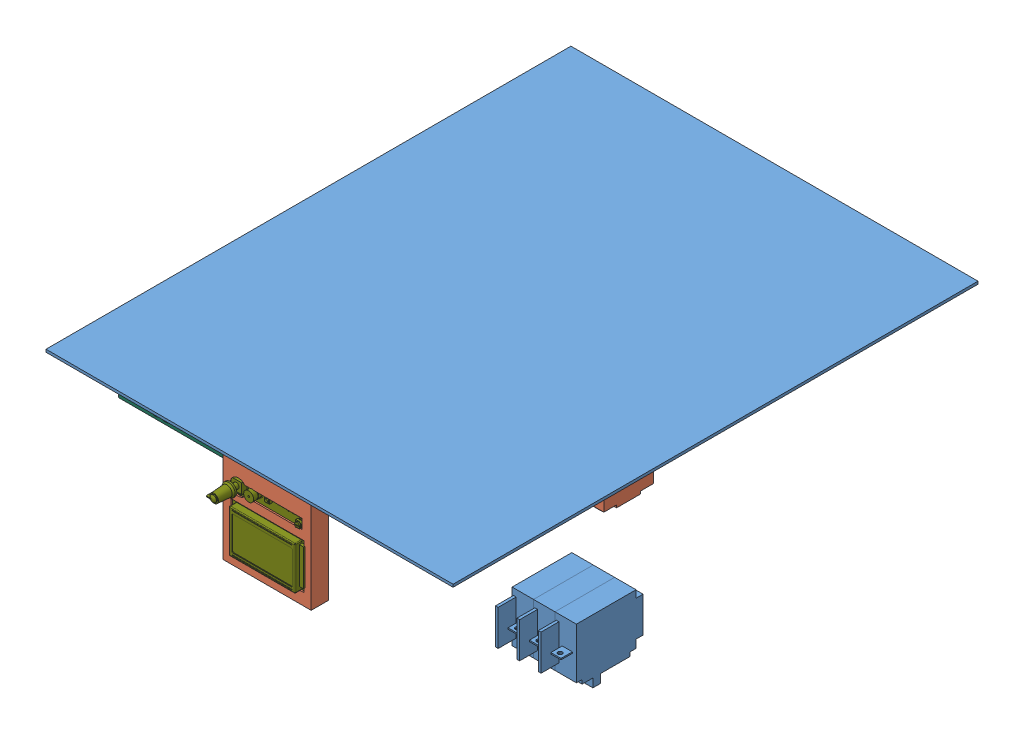
SolidWorks assembly CASE ASSEMBLY, configuration Default. Lengths in mm. (continued)
Components (placement in the parent): (continued)
- BIGTREETECH SKR 2-3D.step-2: BIGTREETECH SKR 2-3D.step [Default] at (122.8656 -8.0191 -250.7922) x (0 0 1) z (0 -1 0) size (112.33 85.75 22.11) (continued)
  - R42.step-1: R42.step [Default] at origin size (1.6 0.8 0.45)
    - R0603.step-1: R0603.step [Default] at (391.1973 179.6035 0) x (1 0 0) z (0 0 1) size (1.6 0.8 0.45)
  - R46.step-1: R46.step [Default] at origin size (0.8 1.6 0.45)
    - R0603.step-1: R0603.step [Default] at (425.1768 173.2653 0) x (0 1 0) z (0 0 1) size (1.6 0.8 0.45)
  - R48.step-1: R48.step [Default] at origin size (1.6 0.8 0.45)
    - R0603.step-1: R0603.step [Default] at (402.9463 182.6842 0) x (1 0 0) z (0 0 1) size (1.6 0.8 0.45)
  - R49.step-1: R49.step [Default] at origin size (0.8 1.6 0.45)
    - R0603.step-1: R0603.step [Default] at (446.7668 160.3113 0) x (0 1 0) z (0 0 1) size (1.6 0.8 0.45)
  - R50.step-1: R50.step [Default] at origin size (0.8 1.6 0.45)
    - R0603.step-1: R0603.step [Default] at (433.2882 166.9697 0) x (0 -1 0) z (0 0 1) size (1.6 0.8 0.45)
  - R52.step-1: R52.step [Default] at origin size (0.8 1.6 0.45)
    - R0603.step-1: R0603.step [Default] at (434.7018 167.0423 0) x (0 1 0) z (0 0 1) size (1.6 0.8 0.45)
  - R53.step-1: R53.step [Default] at origin size (0.8 1.6 0.45)
    - R0603.step-1: R0603.step [Default] at (446.7668 163.3593 0) x (0 1 0) z (0 0 1) size (1.6 0.8 0.45)
  - R54.step-1: R54.step [Default] at origin size (1.6 0.8 0.45)
    - R0603.step-1: R0603.step [Default] at (433.9247 169.8598 0) x (-1 0 0) z (0 0 1) size (1.6 0.8 0.45)
  - R56.step-1: R56.step [Default] at origin size (1.6 0.8 0.45)
    - R0603.step-1: R0603.step [Default] at (433.5407 202.6728 0) x (-1 0 0) z (0 0 1) size (1.6 0.8 0.45)
  - R57.step-1: R57.step [Default] at origin size (1.6 0.8 0.45)
    - R0603.step-1: R0603.step [Default] at (446.2067 202.0128 0) x (-1 0 0) z (0 0 1) size (1.6 0.8 0.45)
  - R58.step-1: R58.step [Default] at origin size (1.6 0.8 0.45)
    - R0603.step-1: R0603.step [Default] at (433.5087 201.1282 0) x (-1 0 0) z (0 0 1) size (1.6 0.8 0.45)
  - R59.step-1: R59.step [Default] at origin size (1.6 0.8 0.45)
    - R0603.step-1: R0603.step [Default] at (446.2816 200.6068 0) x (1 0 0) z (0 0 1) size (1.6 0.8 0.45)
  - R60.step-1: R60.step [Default] at origin size (1.6 0.8 0.45)
    - R0603.step-1: R0603.step [Default] at (398.6873 207.4379 0) x (1 0 0) z (0 0 1) size (1.6 0.8 0.45)
  - R61.step-1: R61.step [Default] at origin size (1.6 0.8 0.45)
    - R0603.step-1: R0603.step [Default] at (402.6377 207.2995 0) x (-1 0 0) z (0 0 1) size (1.6 0.8 0.45)
  - R62.step-1: R62.step [Default] at origin size (1.6 0.8 0.45)
    - R0603.step-1: R0603.step [Default] at (433.5027 199.6398 0) x (-1 0 0) z (0 0 1) size (1.6 0.8 0.45)
  - R64.step-1: R64.step [Default] at origin size (1.6 0.8 0.45)
    - R0603.step-1: R0603.step [Default] at (402.7123 205.8629 0) x (1 0 0) z (0 0 1) size (1.6 0.8 0.45)
  - R70.step-1: R70.step [Default] at origin size (1.6 0.8 0.45)
    - R0603.step-1: R0603.step [Default] at (398.8373 198.8192 0) x (1 0 0) z (0 0 1) size (1.6 0.8 0.45)
  - R71.step-1: R71.step [Default] at origin size (1.6 0.8 0.45)
    - R0603.step-1: R0603.step [Default] at (402.9123 198.7442 0) x (1 0 0) z (0 0 1) size (1.6 0.8 0.45)
  - R73.step-1: R73.step [Default] at origin size (1.6 0.8 0.45)
    - R0603.step-1: R0603.step [Default] at (402.9373 197.2645 0) x (1 0 0) z (0 0 1) size (1.6 0.8 0.45)
  - R75.step-1: R75.step [Default] at origin size (1.6 0.8 0.45)
    - R0603.step-1: R0603.step [Default] at (414.6557 183.6875 0) x (1 0 0) z (0 0 1) size (1.6 0.8 0.45)
  - R76.step-1: R76.step [Default] at origin size (1.6 0.8 0.45)
    - R0603.step-1: R0603.step [Default] at (417.6657 183.6228 0) x (-1 0 0) z (0 0 1) size (1.6 0.8 0.45)
  - R78.step-1: R78.step [Default] at origin size (1.6 0.8 0.45)
    - R0603.step-1: R0603.step [Default] at (417.6657 185.1468 0) x (-1 0 0) z (0 0 1) size (1.6 0.8 0.45)
  - R79.step-1: R79.step [Default] at origin size (1.6 0.8 0.45)
    - R0603.step-1: R0603.step [Default] at (410.1103 163.3762 0) x (1 0 0) z (0 0 1) size (1.6 0.8 0.45)
  - R80.step-1: R80.step [Default] at origin size (0.8 1.6 0.45)
    - R0603.step-1: R0603.step [Default] at (410.8445 159.5197 0) x (0 -1 0) z (0 0 1) size (1.6 0.8 0.45)
  - R81.step-1: R81.step [Default] at origin size (1.6 0.8 0.45)
    - R0603.step-1: R0603.step [Default] at (414.9294 190.8632 0) x (1 0 0) z (0 0 1) size (1.6 0.8 0.45)
  - R82.step-1: R82.step [Default] at origin size (1.6 0.8 0.45)
    - R0603.step-1: R0603.step [Default] at (418.3337 195.4355 0) x (-1 0 0) z (0 0 1) size (1.6 0.8 0.45)
  - R83.step-1: R83.step [Default] at origin size (0.8 1.6 0.45)
    - R0603.step-1: R0603.step [Default] at (409.3632 159.5197 0) x (0 -1 0) z (0 0 1) size (1.6 0.8 0.45)
  - R84.step-1: R84.step [Default] at origin size (1.6 0.8 0.45)
    - R0603.step-1: R0603.step [Default] at (418.3337 193.9418 0) x (-1 0 0) z (0 0 1) size (1.6 0.8 0.45)
  - U4.step-1: U4.step [Default] at origin size (6.2 5 1.75)
    - HSOP8.step-1: HSOP8.step [Default] at (423.1921 177.6994 0) x (1 0 0) z (0 -1 0) size (6.2 1.75 5)
      - Assy_fuss_hsop8_____________.step-1: Assy_fuss_hsop8_____________.step [Default] at (2 0 0) size (1.1 0.95 4.25)
        - Fuss_hsop8_____________.step-1: Fuss_hsop8_____________.step [Default] at (0 0 -0.635) size (1.1 0.95 0.44)
        - Fuss_hsop8_____________.step-2: Fuss_hsop8_____________.step [Default] at (0 0 0.635) size (1.1 0.95 0.44)
        - Fuss_hsop8_____________.step-3: Fuss_hsop8_____________.step [Default] at (0 0 1.905) size (1.1 0.95 0.44)
        - Fuss_hsop8_____________.step-4: Fuss_hsop8_____________.step [Default] at (0 0 -1.905) size (1.1 0.95 0.44)
        - Fuss_hsop8_____________.step-5: Fuss_hsop8_____________.step [Default] at (0 0 -0.635) size (1.1 0.95 0.44)
        - Fuss_hsop8_____________.step-6: Fuss_hsop8_____________.step [Default] at (0 0 0.635) size (1.1 0.95 0.44)
      - Assy_fuss_hsop8_____________-1.step-1: Assy_fuss_hsop8_____________-1.step [Default] at (-2 0 0) x (-1 0 0) z (0 0 -1) size (1.1 0.95 4.25)
        - Fuss_hsop8_____________.step-1: Fuss_hsop8_____________.step [Default] at (0 0 -0.635) size (1.1 0.95 0.44)
        - Fuss_hsop8_____________.step-2: Fuss_hsop8_____________.step [Default] at (0 0 0.635) size (1.1 0.95 0.44)
        - Fuss_hsop8_____________.step-3: Fuss_hsop8_____________.step [Default] at (0 0 1.905) size (1.1 0.95 0.44)
        - Fuss_hsop8_____________.step-4: Fuss_hsop8_____________.step [Default] at (0 0 -1.905) size (1.1 0.95 0.44)
        - Fuss_hsop8_____________.step-5: Fuss_hsop8_____________.step [Default] at (0 0 -0.635) size (1.1 0.95 0.44)
        - Fuss_hsop8_____________.step-6: Fuss_hsop8_____________.step [Default] at (0 0 0.635) size (1.1 0.95 0.44)
      - part_hsop8_____________.step-1: part_hsop8_____________.step [Default] at origin size (4 1.75 5)
  - F1.step-1: F1.step [Default] at origin size (3.48 4.74 1.03)
    - Fuse_1812.step-1: Fuse_1812.step [Default] at (437.3627 175.895 0) x (0 -1 0) z (0 0 1) size (4.73 3.48 1.03)
  - Probe.step-1: Probe.step [Default] at origin size (8 6 11)
    - User_Library-XH2_54_2PIN_RGB0.step-1: User_Library-XH2_54_2PIN_RGB0.step [Default] at (488.1051 165.2532 0) x (-1 0 0) z (0 1 0) size (8 11 6)
  - P1.step-1: P1.step [Default] at origin size (15.24 5.85 7.5)
    - 810112480.step-1: 810112480.step [Default] at (479.9341 168.4042 0) size (15.24 5.84 6)
      - Extruded-31.step-1: Extruded-31.step [Default] at origin size (15.24 5.84 6)
    - 810111120.step-1: 810111120.step [Default] at (485.5337 171.1537 0) size (1.02 0.36 2.4)
      - Extruded-3.step-1: Extruded-3.step [Default] at origin size (1.02 0.36 2.4)
    - 810112616.step-1: 810112616.step [Default] at (480.2983 171.1537 0) size (9.38 0.36 6)
      - Extruded-32.step-1: Extruded-32.step [Default] at origin size (9.38 0.36 6)
    - 810112752.step-1: 810112752.step [Default] at (479.972 168.3823 0) size (14.76 5.32 0.5)
      - Extruded-33.step-1: Extruded-33.step [Default] at origin size (14.76 5.32 0.5)
    - 860059712.step-1: 860059712.step [Default] at (477.402 168.7861 -1.5) x (0 1 0) z (0 0 1) size (1 1 6)
      - Cylinder.step-1: Cylinder.step [Default] at origin size (1 1 6)
    - 860059712.step-2: 860059712.step [Default] at (479.942 168.7861 -1.5) x (0 1 0) z (0 0 1) size (1 1 6)
      - Cylinder.step-1: Cylinder.step [Default] at origin size (1 1 6)
    - 860059712.step-3: 860059712.step [Default] at (482.482 168.7861 -1.5) x (0 1 0) z (0 0 1) size (1 1 6)
      - Cylinder.step-1: Cylinder.step [Default] at origin size (1 1 6)
    - 860059712.step-4: 860059712.step [Default] at (485.022 168.7861 -1.5) x (0 1 0) z (0 0 1) size (1 1 6)
      - Cylinder.step-1: Cylinder.step [Default] at origin size (1 1 6)
    - 810110576.step-1: 810110576.step [Default] at (475.101 171.1382 0) size (1.02 0.37 2.4)
      - Extruded.step-1: Extruded.step [Default] at origin size (1.02 0.37 2.4)
    - 860060864.step-1: 860060864.step [Default] at (474.856 168.9105 0) x (-1 0 0) z (0 0 1) size (1 1 4.5)
      - Cylinder-34.step-1: Cylinder-34.step [Default] at origin size (1 1 4.5)
  - R88.step-1: R88.step [Default] at origin size (1.6 0.8 0.45)
    - R0603.step-1: R0603.step [Default] at (464.0563 185.2452 0) x (1 0 0) z (0 0 1) size (1.6 0.8 0.45)
  - R89.step-1: R89.step [Default] at origin size (1.6 0.8 0.45)
    - R0603.step-1: R0603.step [Default] at (464.0563 186.7202 0) x (1 0 0) z (0 0 1) size (1.6 0.8 0.45)
  - R90.step-1: R90.step [Default] at origin size (1.6 0.8 0.45)
    - R0603.step-1: R0603.step [Default] at (464.0563 188.1952 0) x (1 0 0) z (0 0 1) size (1.6 0.8 0.45)
  - D14.step-1: D14.step [Default] at origin size (1.61 0.81 0.61)
    - LED_0603_G.step-1: LED_0603_G.step [Default] at (443.6801 162.0518 0) x (-1 0 0) z (0 0 1) size (1.61 0.81 0.61)
      - User_Library-LED_0603_G_Pocket002.step-1: User_Library-LED_0603_G_Pocket002.step [Default] at origin size (0.41 0.81 0.21)
      - User_Library-LED_0603_G_Pad004.step-1: User_Library-LED_0603_G_Pad004.step [Default] x (1 0 0) z (0 0 -1) size (0.4 0.8 0)
      - User_Library-LED_0603_G_Fillet.step-1: User_Library-LED_0603_G_Fillet.step [Default] at origin size (1 0.7 0.4)
      - User_Library-LED_0603_G_Pocket001.step-1: User_Library-LED_0603_G_Pocket001.step [Default] at origin size (0.4 0.8 0.2)
      - User_Library-LED_0603_G_Pad.step-1: User_Library-LED_0603_G_Pad.step [Default] at origin size (0.8 0.8 0.2)
  - C21.step-1: C21.step [Default] at origin size (1.6 0.8 0.8)
    - 810108944.step-1: 810108944.step [Default] at (458.6741 172.9827 0) size (1.14 0.8 0.8)
      - Extruded-22.step-1: Extruded-22.step [Default] at origin size (1.14 0.8 0.8)
    - 810108400.step-1: 810108400.step [Default] at (457.9891 172.9826 0) size (0.23 0.8 0.8)
      - Extruded-23.step-1: Extruded-23.step [Default] at origin size (0.23 0.8 0.8)
    - 810108400.step-2: 810108400.step [Default] at (459.3591 172.9826 0) size (0.23 0.8 0.8)
      - Extruded-23.step-1: Extruded-23.step [Default] at origin size (0.23 0.8 0.8)
  - C60.step-1: C60.step [Default] at origin size (2 1.25 0.78)
    - User_Library-0805_SMD_Capacitor.step-1: User_Library-0805_SMD_Capacitor.step [Default] at (458.5985 175.133 -0.01) x (1 0 0) z (0 -1 0) size (2 0.78 1.25)
  - C61.step-1: C61.step [Default] at origin size (0.81 1.6 0.8)
    - 810109216.step-1: 810109216.step [Default] at (458.0803 162.4211 0) size (0.8 1.14 0.8)
      - Extruded-11.step-1: Extruded-11.step [Default] at origin size (0.8 1.14 0.8)
    - 810109080.step-1: 810109080.step [Default] at (458.0804 161.7361 0) size (0.8 0.23 0.8)
      - Extruded-10.step-1: Extruded-10.step [Default] at origin size (0.8 0.23 0.8)
    - 810109080.step-2: 810109080.step [Default] at (458.0804 163.1061 0) size (0.8 0.23 0.8)
      - Extruded-10.step-1: Extruded-10.step [Default] at origin size (0.8 0.23 0.8)
  - C62.step-1: C62.step [Default] at origin size (1.6 0.8 0.8)
    - 810108944.step-1: 810108944.step [Default] at (463.8994 193.9377 0) size (1.14 0.8 0.8)
      - Extruded-22.step-1: Extruded-22.step [Default] at origin size (1.14 0.8 0.8)
    - 810108400.step-1: 810108400.step [Default] at (463.2144 193.9376 0) size (0.23 0.8 0.8)
      - Extruded-23.step-1: Extruded-23.step [Default] at origin size (0.23 0.8 0.8)
    - 810108400.step-2: 810108400.step [Default] at (464.5844 193.9376 0) size (0.23 0.8 0.8)
      - Extruded-23.step-1: Extruded-23.step [Default] at origin size (0.23 0.8 0.8)
  - C63.step-1: C63.step [Default] at origin size (0.8 1.6 0.8)
    - 810109216.step-1: 810109216.step [Default] at (448.5727 199.9859 0) size (0.8 1.14 0.8)
      - Extruded-11.step-1: Extruded-11.step [Default] at origin size (0.8 1.14 0.8)
    - 810109080.step-1: 810109080.step [Default] at (448.5726 200.6709 0) size (0.8 0.23 0.8)
      - Extruded-10.step-1: Extruded-10.step [Default] at origin size (0.8 0.23 0.8)
    - 810109080.step-2: 810109080.step [Default] at (448.5726 199.3009 0) size (0.8 0.23 0.8)
      - Extruded-10.step-1: Extruded-10.step [Default] at origin size (0.8 0.23 0.8)
  - D19.step-1: D19.step [Default] at origin size (1.61 0.81 0.61)
    - LED_0603_G.step-1: LED_0603_G.step [Default] at (414.9232 199.3538 0) x (-1 0 0) z (0 0 1) size (1.61 0.81 0.61)
      - User_Library-LED_0603_G_Pocket002.step-1: User_Library-LED_0603_G_Pocket002.step [Default] at origin size (0.41 0.81 0.21)
      - User_Library-LED_0603_G_Pad004.step-1: User_Library-LED_0603_G_Pad004.step [Default] x (1 0 0) z (0 0 -1) size (0.4 0.8 0)
      - User_Library-LED_0603_G_Fillet.step-1: User_Library-LED_0603_G_Fillet.step [Default] at origin size (1 0.7 0.4)
      - User_Library-LED_0603_G_Pocket001.step-1: User_Library-LED_0603_G_Pocket001.step [Default] at origin size (0.4 0.8 0.2)
      - User_Library-LED_0603_G_Pad.step-1: User_Library-LED_0603_G_Pad.step [Default] at origin size (0.8 0.8 0.2)
  - D20.step-1: D20.step [Default] at origin size (1.25 2.02 1.1)
    - User_Library-led_0805.step-1: User_Library-led_0805.step [Default] at (462.7879 175.6538 0) x (0 1 0) z (0 0 1) size (2.02 1.25 1.1)
  - J1.step-1: J1.step [Default] at origin size (12.7 2.54 11.54)
    - 1001-5.step-1: 1001-5.step [Default] at (468.874 170.561 0) x (-1 0 0) z (0 0 1) size (12.7 2.54 11.54)
  - P2.step-1: P2.step [Default] at origin size (5.08 7.62 11.54)
    - 1001-3.step-1: 1001-3.step [Default] at (452.9366 163.9727 0) x (0 1 0) z (0 0 1) size (7.62 2.54 11.54)
    - 1001-3.step-2: 1001-3.step [Default] at (455.4766 163.9727 0) x (0 1 0) z (0 0 1) size (7.62 2.54 11.54)
  - Q10.step-1: Q10.step [Default] at origin size (3 3 1.3)
    - 860057152.step-1: 860057152.step [Default] at (414.6295 201.7671 0) x (0 -1 0) z (-1 0 0) size (3 1.3 3)
  - R16.step-1: R16.step [Default] at origin size (1.6 0.8 0.45)
    - R0603.step-1: R0603.step [Default] at (465.2907 172.9548 0) x (-1 0 0) z (0 0 1) size (1.6 0.8 0.45)
  - R18.step-1: R18.step [Default] at origin size (0.8 1.6 0.45)
    - R0603.step-1: R0603.step [Default] at (461.2448 175.6724 0) x (0 1 0) z (0 0 1) size (1.6 0.8 0.45)
  - R19.step-1: R19.step [Default] at origin size (1.6 0.8 0.45)
    - R0603.step-1: R0603.step [Default] at (462.0633 172.9932 0) x (1 0 0) z (0 0 1) size (1.6 0.8 0.45)
  - R45.step-1: R45.step [Default] at origin size (1.6 0.8 0.45)
    - R0603.step-1: R0603.step [Default] at (455.7657 161.6518 0) x (-1 0 0) z (0 0 1) size (1.6 0.8 0.45)
  - R47.step-1: R47.step [Default] at origin size (1.6 0.8 0.45)
    - R0603.step-1: R0603.step [Default] at (452.7923 161.6902 0) x (1 0 0) z (0 0 1) size (1.6 0.8 0.45)
  - R85.step-1: R85.step [Default] at origin size (0.8 1.6 0.45)
    - R0603.step-1: R0603.step [Default] at (432.2065 162.8147 0) x (0 -1 0) z (0 0 1) size (1.6 0.8 0.45)
  - R92.step-1: R92.step [Default] at origin size (1.6 0.8 0.45)
    - R0603.step-1: R0603.step [Default] at (414.9294 197.8492 0) x (1 0 0) z (0 0 1) size (1.6 0.8 0.45)
  - R93.step-1: R93.step [Default] at origin size (1.6 0.8 0.45)
    - R0603.step-1: R0603.step [Default] at (418.2897 202.5098 0) x (-1 0 0) z (0 0 1) size (1.6 0.8 0.45)
  - R94.step-1: R94.step [Default] at origin size (1.6 0.8 0.45)
    - R0603.step-1: R0603.step [Default] at (418.2897 200.9858 0) x (-1 0 0) z (0 0 1) size (1.6 0.8 0.45)
  - U1.step-1: U1.step [Default] at origin size (14 14 1.15)
    - 810113568.step-1: 810113568.step [Default] at (451.7654 188.208 0.05) size (14 14 1.15)
      - Extruded-35.step-1: Extruded-35.step [Default] at origin size (14 14 1.15)
  - Y1.step-1: Y1.step [Default] at origin size (3.21 2.5 0.81)
    - 810113840.step-1: 810113840.step [Default] at (451.358 176.149 0.15) size (2.8 2.1 0.66)
      - Extruded-36.step-1: Extruded-36.step [Default] at origin size (2.8 2.1 0.66)
    - User_Library-GeyerElectronics_KX7.step-1: User_Library-GeyerElectronics_KX7.step [Default] at (451.3649 176.1489 0) x (1 0 0) z (0 -1 0) size (3.21 0.81 2.5)
  - C42.step-1: C42.step [Default] at origin size (6.6 7 5.2)
    - SL-E.step-1: SL-E.step [Default] at (414.6551 167.817 0) x (0 -1 0) z (0 0 1) size (7 6.6 5.2)
  - C28.step-1: C28.step [Default] at origin size (0.81 1.6 0.8)
    - 810109216.step-1: 810109216.step [Default] at (406.6183 171.2731 0) size (0.8 1.14 0.8)
      - Extruded-11.step-1: Extruded-11.step [Default] at origin size (0.8 1.14 0.8)
    - 810109080.step-1: 810109080.step [Default] at (406.6184 170.5881 0) size (0.8 0.23 0.8)
      - Extruded-10.step-1: Extruded-10.step [Default] at origin size (0.8 0.23 0.8)
    - 810109080.step-2: 810109080.step [Default] at (406.6184 171.9581 0) size (0.8 0.23 0.8)
      - Extruded-10.step-1: Extruded-10.step [Default] at origin size (0.8 0.23 0.8)
  - Board.step-1: Board.step [Default] at (0 0 -0.9449) size (109.66 84.3 0.94)
- RaspberryPi2 STEP214-1: RaspberryPi2 STEP214 [Default] at (26.0933 -8.3742 261.8958) x (0 0 -1) z (-1 0 0) size (89.62 18.75 58.3)
  - Mainboard2.STEP-1: Mainboard2.STEP [Default] at origin size (85 1.3 56)
  - GPIO.STEP-1: GPIO.STEP [Default] at (-11.37 0 -24.5) x (0 0 1) z (-1 0 0) size (5 11.5 50.8)
  - Processor.STEP-1: Processor.STEP [Default] at (-15.5 0 -3) x (0 0 1) z (-1 0 0) size (14 1 14)
  - GPU.STEP-1: GPU.STEP [Default] at (15.25 0 -5.75) x (0 0 1) z (-1 0 0) size (9.1 1 9.1)
  - CameraAssembly.STEP-1: CameraAssembly.STEP [Default] at (10.0885 -2.9159 16.55) x (-1 0 0) z (0 0 -1) size (5.01 5.51 22.11)
  - CameraAssembly.STEP-2: CameraAssembly.STEP [Default] at (-46.3885 -2.9159 0) size (5.01 5.51 22.11)
  - HDMI.STEP-1: HDMI.STEP [Default] at (-10.2 0.27 29.3) size (15.04 8.38 12.15)
  - RAM.STEP-1: RAM.STEP [Default] at (0.5 -2.3 -6) x (0 0 1) z (-1 0 0) size (12 1 12)
  - Audio.STEP-1: Audio.STEP [Default] at (10.9 0.15 21.75) size (7 6 14.8)
  - MicroSDSocket.STEP-1: MicroSDSocket.STEP [Default] at (-34.5 -1.3 -0.7) x (0 0 -1) z (-1 0 0) size (13 1.3 14)
  - MicroSD.STEP-1: MicroSD.STEP [Default] at (-37 -2.3 0.1) x (0 0 1) z (-1 0 0) size (11.01 1 15)
  - micro USB2.STEP-1: micro USB2.STEP [Default] at (-17.2704 -5.0969 44.9026) size (7.98 2.93 5.58)
  - usb double.STEP-1: usb double.STEP [Default] at (30.38 -0.09 -18.85) x (0 0 -1) z (1 0 0) size (15.6 18.75 17.92)
  - usb double.STEP-2: usb double.STEP [Default] at (30.38 -0.09 -1.25) x (0 0 -1) z (1 0 0) size (15.6 18.75 17.92)
  - RJ45-LED.STEP-1: RJ45-LED.STEP [Default] at (34.11 7.4 17.348) x (1 0 0) z (0 -1 0) size (21.3 18 14.1)
- WELL RSP500-48 POWER SUPPLY-1: WELL RSP500-48 POWER SUPPLY [Default] at (-192.2085 2.1008 190.5974) x (0 0 1) z (1 0 0) size (230 40.51 127)
- RepRapDiscount_Full Graphic Smart Controller-1: RepRapDiscount_Full Graphic Smart Controller [Valor predeterminado] at (-67.6302 -82.5522 309.3738) x (-1 0 0) z (0 0 1) size (93 87.2 45.8)
- Buck Converter 1-1: Buck Converter 1 [Default] at (90.8108 -7.0742 287.9672) x (0 0 1) z (1 0 0) size (43.76 13.72 30.51)
- Buck Converter 2-1: Buck Converter 2 [Default] at (113.4295 -7.0742 205.1378) x (-1 0 0) z (0 0 1) size (53.8 17.5 23.88)
- Breaker-1: Breaker [Default] at (289.2121 48.8318 348.7765) x (0 0 1) z (1 0 0) size (100.28 75.18 76.2)
  - Breaker Component-1: Breaker Component [Default] at origin size (100.28 75.18 25.4)
  - Breaker Component-2: Breaker Component [Default] at (0 0 25.4) size (100.28 75.18 25.4)
  - Breaker Component-3: Breaker Component [Default] at (0 0 50.8) size (100.28 75.18 25.4)
- Buck Converter 1-2: Buck Converter 1 [Default] at (134.0162 -7.0742 287.9801) x (0 0 1) z (1 0 0) size (43.76 13.72 30.51)
- Buck Converter 2-2: Buck Converter 2 [Default] at (113.4295 -7.0742 241.7138) x (-1 0 0) z (0 0 1) size (53.8 17.5 23.88)
- SSR--H1.step-2: SSR--H1.step [Default] at (22.4153 -7.0742 117.6478) x (0 0 -1) z (-1 0 0) size (58.7 23.5 45.2)
- SSR--H1.step-3: SSR--H1.step [Default] at (138.2153 -7.0742 117.6478) x (0 0 -1) z (-1 0 0) size (58.7 23.5 45.2)
- side-1: side [Default] at (-298.6347 -64.5742 126.6518) x (0 0 -1) z (-1 0 0) size (381 133.35 3.17) (hidden)
- front-1: front [Default] at (-63.6847 -64.5742 313.9768) x (-1 0 0) z (0 0 1) size (469.9 133.35 3.17) (hidden)
- side-2: side [Default] at (171.2653 -64.5742 126.6518) x (0 0 -1) z (1 0 0) size (381 133.35 3.17) (hidden)
- lcd display case-1: lcd display case [Default] at (-68.3837 -66.0982 281.0838) x (-1 0 0) z (0 0 1) size (104.65 130.05 36.07)
- back-1: back [Default] at (-63.6847 -64.5742 -67.0232) size (469.9 133.35 3.17) (hidden)
- top-1: top [Default] at (-63.6847 -131.2492 126.6518) x (1 0 0) z (0 -1 0) size (469.9 381 3.17) (hidden)
- 11.12X11.2-1: 11.12X11.2 [Default] at (14.9283 2.1008 196.3748) x (-1 0 0) z (0 0 1) size (287.27 41.27 241.55)
Mates (geometry in assembly coordinates):
- Coincident1: coincident anti-aligned: plane of 24.5x24 sheet metal-1 through (-63.6847 2.1008 31.4018) normal (0 -1 0); plane of WELL RSP500-48 POWER SUPPLY-1 through (-192.2085 2.1008 190.5974) normal (0 1 0)
- Distance17: distance = 12.7 mm: plane of Buck Converter 2-1 through (140.3281 -8.522 217.0758) normal (0 0 1); line of Buck Converter 2-2 through (140.3281 -7.0742 229.7758) axis (-1 0 0)
- Distance31: distance = 12.7 mm anti-aligned: plane of SSR--H1.step-1 through (57.7153 -26.9742 146.9978) normal (-1 0 0); plane of SSR--H1.step-2 through (45.0153 -26.9742 146.9978) normal (1 0 0)
- Distance30: distance = 12.7 mm anti-aligned: plane of SSR--H1.step-1 through (102.9153 -26.9742 146.9978) normal (1 0 0); plane of SSR--H1.step-3 through (115.6153 -26.9742 146.9978) normal (-1 0 0)
- Distance18: distance = 304.8 mm: plane of SSR--H1.step-2 through (-0.1847 -26.9742 146.9978) normal (-1 0 0); line of 24.5x24 sheet metal-1 through (-304.9847 5.2758 -279.7482) axis (0 0 1)
- Distance28: distance = 3.175 mm aligned: plane of side-1 through (-301.8097 -64.5742 126.6518) normal (-1 0 0); plane of 24.5x24 sheet metal-1 through (-304.9847 5.2758 342.5518) normal (-1 0 0)
- Coincident46: coincident anti-aligned: plane of 24.5x24 sheet metal-1 through (-63.6847 2.1008 31.4018) normal (0 -1 0); plane of side-1 through (-301.8097 2.1008 317.1518) normal (0 1 0)
- Distance27: distance = 25.4 mm aligned: plane of 24.5x24 sheet metal-1 through (-304.9847 5.2758 342.5518) normal (0 0 1); plane of side-1 through (-301.8097 2.1008 317.1518) normal (0 0 1)
- Distance32: distance = 25.4 mm aligned: plane of front-1 through (-63.6847 -64.5742 317.1518) normal (0 0 1); plane of 24.5x24 sheet metal-1 through (-304.9847 5.2758 342.5518) normal (0 0 1)
- Coincident58: coincident aligned: plane of side-1 through (-301.8097 2.1008 -63.8482) normal (0 0 -1); plane of side-2 through (174.4403 -131.2492 -63.8482) normal (0 0 -1)
- Distance33: distance = 3.175 mm aligned: plane of side-2 through (174.4403 -64.5742 126.6518) normal (1 0 0); plane of 24.5x24 sheet metal-1 through (177.6153 5.2758 342.5518) normal (1 0 0)
- Coincident60: coincident anti-aligned: plane of 24.5x24 sheet metal-1 through (-63.6847 2.1008 31.4018) normal (0 -1 0); plane of side-2 through (174.4403 2.1008 317.1518) normal (0 1 0)
- Coincident61: coincident anti-aligned: plane of 24.5x24 sheet metal-1 through (-63.6847 2.1008 31.4018) normal (0 -1 0); plane of front-1 through (171.2653 2.1008 317.1518) normal (0 1 0)
- Coincident62: coincident anti-aligned: plane of front-1 through (171.2653 2.1008 317.1518) normal (1 0 0); plane of side-2 through (171.2653 -64.5742 126.6518) normal (-1 0 0)
- Distance67: distance = 3.175 mm anti-aligned: plane of 24.5x24 sheet metal-1 through (-63.6847 2.1008 31.4018) normal (0 -1 0); plane of lcd display case-1 through (-16.0597 -1.0742 317.1518) normal (0 1 0)
- Distance36: distance = 6.35 mm anti-aligned: plane of front-1 through (-9.7097 2.1008 313.9768) normal (-1 0 0); plane of lcd display case-1 through (-16.0597 -1.0742 317.1518) normal (1 0 0)
- Coincident65: coincident anti-aligned: plane of RepRapDiscount_Full Graphic Smart Controller-1 through (-67.6302 -82.5522 315.3738) normal (0 0 1); plane of lcd display case-1 through (-68.3837 -66.0982 315.3738) normal (0 0 -1)
- Coincident66: coincident anti-aligned: plane of RepRapDiscount_Full Graphic Smart Controller-1 through (-28.6302 -117.1522 323.6738) normal (0 -1 0); plane of lcd display case-1 through (-110.9262 -117.1522 298.3558) normal (0 1 0)
- Distance37: distance = 4.064 mm anti-aligned: plane of RepRapDiscount_Full Graphic Smart Controller-1 through (-28.6302 -117.1522 323.6738) normal (1 0 0); plane of lcd display case-1 through (-24.5662 -117.1522 298.3558) normal (-1 0 0)
- Coincident68: coincident aligned: plane of front-1 through (-63.6847 -64.5742 317.1518) normal (0 0 1); plane of lcd display case-1 through (-68.3837 -66.0982 317.1518) normal (0 0 1)
- Coincident69: coincident anti-aligned: plane of side-1 through (-301.8097 2.1008 -63.8482) normal (0 0 -1); plane of back-1 through (-63.6847 -64.5742 -63.8482) normal (0 0 1)
- Coincident70: coincident aligned: plane of front-1 through (-298.6347 2.1008 317.1518) normal (-1 0 0); plane of back-1 through (-298.6347 -131.2492 -63.8482) normal (-1 0 0)
- Coincident71: coincident aligned: plane of side-1 through (-301.8097 -131.2492 317.1518) normal (0 -1 0); plane of back-1 through (-298.6347 -131.2492 -63.8482) normal (0 -1 0)
- Coincident96: coincident anti-aligned: plane of side-1 through (-301.8097 -131.2492 317.1518) normal (0 -1 0); plane of top-1 through (-63.6847 -131.2492 126.6518) normal (0 1 0)
- Coincident97: coincident anti-aligned: plane of back-1 through (-63.6847 -64.5742 -63.8482) normal (0 0 1); plane of top-1 through (-298.6347 -134.4242 -63.8482) normal (0 0 -1)
- Coincident98: coincident anti-aligned: plane of side-2 through (171.2653 -64.5742 126.6518) normal (-1 0 0); plane of top-1 through (171.2653 -134.4242 -63.8482) normal (1 0 0)
- Distance54: distance = 12.7 mm anti-aligned: plane of Buck Converter 1-1 through (106.1575 -8.6617 287.9672) normal (1 0 0); plane of Buck Converter 1-2 through (118.8575 -8.6617 287.9801) normal (-1 0 0)
- Coincident101: coincident anti-aligned: plane of 24.5x24 sheet metal-1 through (-63.6847 2.1008 31.4018) normal (0 -1 0); plane of 11.12X11.2-1 through (14.9283 2.1008 196.3748) normal (0 1 0)
- Distance56: distance = 19.05 mm aligned: plane of 11.12X11.2-1 through (158.5653 -1.0742 317.1518) normal (1 0 0); plane of 24.5x24 sheet metal-1 through (177.6153 5.2758 342.5518) normal (1 0 0)
- Distance60: distance = 12.7 mm aligned: plane of SSR--H1.step-1 through (102.9153 -26.9742 88.2978) normal (0 0 -1); plane of 11.12X11.2-1 through (158.5653 -1.0742 75.5978) normal (0 0 -1)
- Coincident108: coincident aligned: plane of SSR--H1.step-1 through (102.9153 -26.9742 88.2978) normal (0 0 -1); plane of SSR--H1.step-2 through (45.0153 -26.9742 88.2978) normal (0 0 -1)
- Coincident109: coincident aligned: plane of SSR--H1.step-1 through (102.9153 -26.9742 88.2978) normal (0 0 -1); plane of SSR--H1.step-3 through (160.8153 -26.9742 88.2978) normal (0 0 -1)
- Distance61: distance = 63.5 mm aligned: plane of Buck Converter 2-2 through (140.3281 -8.522 253.6518) normal (0 0 1); plane of 11.12X11.2-1 through (158.5653 -1.0742 317.1518) normal (0 0 1)
- Coincident115: coincident aligned: plane of Buck Converter 2-1 through (140.3281 -8.522 217.0758) normal (1 0 0); plane of Buck Converter 2-2 through (140.3281 -8.522 253.6518) normal (1 0 0)
- Coincident119: coincident aligned: plane of lcd display case-1 through (-68.3837 -66.0982 317.1518) normal (0 0 1); plane of 11.12X11.2-1 through (158.5653 -1.0742 317.1518) normal (0 0 1)
- Coincident120: coincident: plane of WELL RSP500-48 POWER SUPPLY-1 through (-128.7087 -38.3991 305.5971) normal (1 0 0); line of 11.12X11.2-1 through (-128.7087 -1.0742 317.1518) axis (0 0 -1)
- Coincident121: coincident aligned: plane of WELL RSP500-48 POWER SUPPLY-1 through (-255.7083 -38.3991 75.5978) normal (0 0 -1); plane of 11.12X11.2-1 through (158.5653 -1.0742 75.5978) normal (0 0 -1)
- Coincident122: coincident anti-aligned: plane of RaspberryPi2 STEP214-1/Mainboard2.STEP-1 through (0.5933 -7.0742 221.8958) normal (0 1 0); plane of 11.12X11.2-1 through (50.6153 -7.0742 300.8958) normal (0 -1 0)
- Coincident123: coincident anti-aligned: plane of BIGTREETECH SKR 2-3D.step-2/Board.step-1 through (-26.2324 -7.0742 138.4374) normal (0 1 0); plane of 11.12X11.2-1 through (14.9283 -7.0742 196.3748) normal (0 -1 0)
- Concentric2: concentric aligned: cylinder of BIGTREETECH SKR 2-3D.step-2/Board.step-1 through (-29.0137 -7.0742 142.3998) axis (0 1 0) radius 1.7272; cylinder of 11.12X11.2-1 through (-29.0137 -7.0742 142.3998) axis (0 1 0) radius 1.5
- Coincident124: coincident anti-aligned: plane of SSR--H1.step-1 through (80.3153 -7.0742 117.6478) normal (0 1 0); plane of 11.12X11.2-1 through (14.9283 -7.0742 196.3748) normal (0 -1 0)
- Coincident125: coincident aligned: plane of SSR--H1.step-1 through (80.3153 -30.0742 117.6478) normal (0 -1 0); plane of SSR--H1.step-2 through (22.4153 -30.0742 117.6478) normal (0 -1 0)
- Coincident126: coincident aligned: plane of SSR--H1.step-1 through (80.3153 -30.0742 117.6478) normal (0 -1 0); plane of SSR--H1.step-3 through (138.2153 -30.0742 117.6478) normal (0 -1 0)
- Coincident127: coincident anti-aligned: plane of Buck Converter 1-1 through (90.8108 -7.0742 287.9672) normal (0 1 0); plane of 11.12X11.2-1 through (102.4313 -7.0742 305.9758) normal (0 -1 0)
- Coincident128: coincident anti-aligned: plane of Buck Converter 2-1 through (113.4295 -7.0742 205.1378) normal (0 1 0); plane of 11.12X11.2-1 through (118.1793 -7.0742 195.7398) normal (0 -1 0)
- Concentric5: concentric aligned: cylinder of Buck Converter 1-1 through (102.4313 -8.6617 305.9758) axis (0 1 0) radius 1.5875; cylinder of 11.12X11.2-1 through (102.4313 -7.0742 305.9758) axis (0 1 0) radius 1.5
- Coincident131: coincident aligned: plane of Buck Converter 2-1 through (113.4295 -8.522 205.1378) normal (0 -1 0); plane of Buck Converter 2-2 through (113.4295 -8.522 241.7138) normal (0 -1 0)
- Concentric3: concentric anti-aligned: cylinder of RaspberryPi2 STEP214-1/Mainboard2.STEP-1 through (1.5933 -7.0742 300.8958) axis (0 -1 0) radius 1.25; cylinder of 11.12X11.2-1 through (1.5933 -7.0742 300.8958) axis (0 1 0) radius 1.5
- Coincident132: coincident anti-aligned: plane of RaspberryPi2 STEP214-1/Mainboard2.STEP-1 through (0.5933 -7.0742 221.8958) normal (0 1 0); plane of 11.12X11.2-1 through (1.5933 -7.0742 300.8958) normal (0 -1 0)
